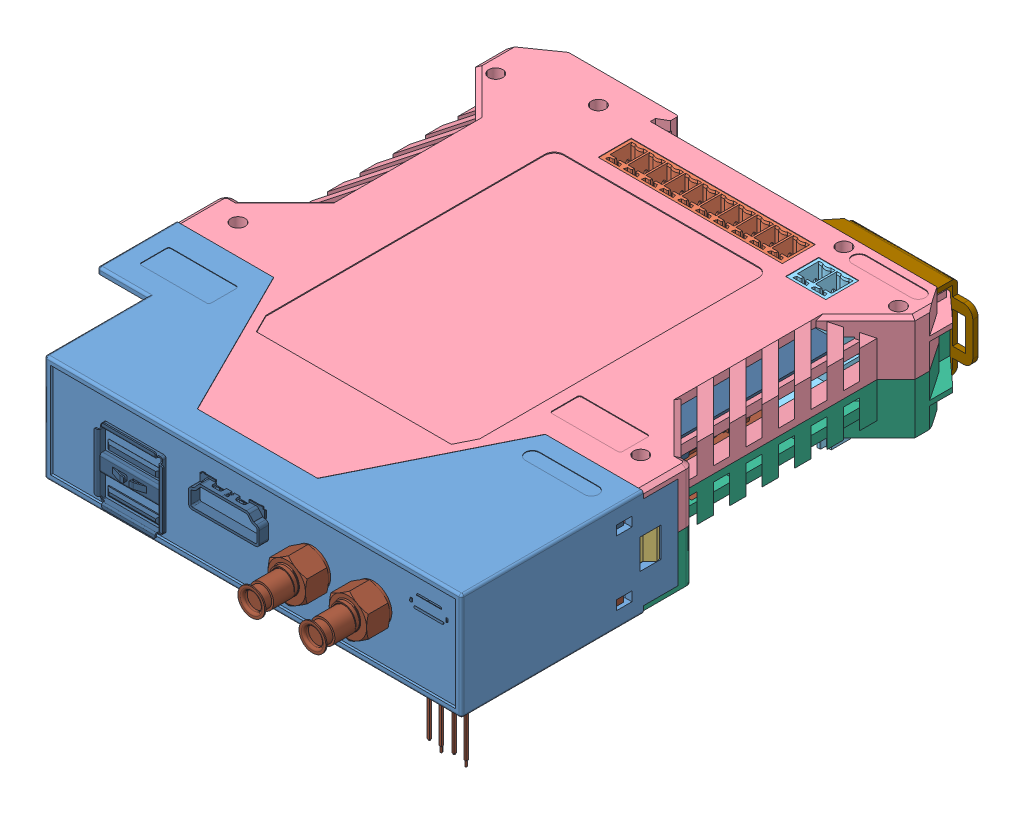
SolidWorks assembly 22.5-rasp, configuration По умолчанию. Lengths in mm.
Overall size (99 35.36 126.04).
16 component instances, 16 part files, 5 mates.
Components (placement in the parent):
- 2019_05_09__13-53-04-633-1: 2019_05_09__13-53-04-633 [По умолчанию] at origin size (88.8 1.5 44.9) (hidden)
- 2019_05_09__13-53-04-602-1: 2019_05_09__13-53-04-602 [По умолчанию] at origin size (80 1.5 47.15) (hidden)
- 2019_05_09__13-53-04-570-1: 2019_05_09__13-53-04-570 [По умолчанию] at origin size (80 1.5 21.25) (hidden)
- 2019_05_09__13-53-04-539-1: 2019_05_09__13-53-04-539 [По умолчанию] at origin size (13.2 1.5 24.9) (hidden)
- 2019_05_09__13-53-04-508-1: 2019_05_09__13-53-04-508 [По умолчанию] at origin size (15.55 19.95 18) (hidden)
- 2019_05_09__13-53-04-477-1: 2019_05_09__13-53-04-477 [По умолчанию] at origin size (99 22.6 45.85)
- 2019_05_09__13-53-04-445-1: 2019_05_09__13-53-04-445 [По умолчанию] at origin size (41 29 18.7)
- 2019_05_09__13-53-04-414-1: 2019_05_09__13-53-04-414 [По умолчанию] at origin size (2.65 10 10.5)
- 2019_05_09__13-53-04-383-1: 2019_05_09__13-53-04-383 [По умолчанию] at origin size (99 16.3 106.2)
- 2019_05_09__13-53-04-352-1: 2019_05_09__13-53-04-352 [По умолчанию] at origin size (10.52 29 18.6)
- 2019_05_09__13-53-04-320-1: 2019_05_09__13-53-04-320 [По умолчанию] at origin size (99 11.3 106.2)
- 2019_05_09__13-53-04-289-1: 2019_05_09__13-53-04-289 [По умолчанию] at origin size (2.65 10 10.5)
- 2019_05_09__13-53-04-258-1: 2019_05_09__13-53-04-258 [По умолчанию] at origin size (9.5 5 15.25)
- 2019_05_09__13-53-04-227-1: 2019_05_09__13-53-04-227 [По умолчанию] at origin size (30 17.5 6.6)
- XXXX.687253.006-1: XXXX.687253.006 [По умолчанию] at (47.65 19.1 105.4417) x (1 0 0) z (0 1 0) size (88.8 94.05 20.2)
- XXXX.687253.007-1: XXXX.687253.007 [По умолчанию] at (-11.05 5.0914 105.4417) x (1 0 0) z (0 1 0) size (88.8 113.3 33.84)
Mates (geometry in assembly coordinates):
- Расстояние1: distance = 0.2 mm anti-aligned: plane of XXXX.687253.007-1 through (39.95 3.5 68.5417) normal (1 0 0); plane of 2019_05_09__13-53-04-320-1 through (40.15 8.8 68.5) normal (-1 0 0)
- Совпадение3: coincident anti-aligned: plane of 2019_05_09__13-53-04-320-1 through (0.55 3.5 68.5) normal (0 1 0); plane of XXXX.687253.007-1 through (-36.55 3.5 71.9417) normal (0 -1 0)
- Совпадение4: coincident aligned: plane of XXXX.687253.006-1 through (47.65 17.6237 105.4417) normal (0 0 1); plane of XXXX.687253.007-1 through (47.65 3.5 105.4417) normal (0 0 1)
- Совпадение5: coincident anti-aligned: plane of 2019_05_09__13-53-04-383-1 through (-0.55 19.1 68.4902) normal (0 -1 0); plane of XXXX.687253.006-1 through (-37.05 19.1 105.4417) normal (0 1 0)
- Расстояние2: distance = 0.2 mm anti-aligned: plane of XXXX.687253.006-1 through (39.95 17.6237 16.8917) normal (1 0 0); plane of 2019_05_09__13-53-04-383-1 through (40.15 16.3 14.4902) normal (-1 0 0)
